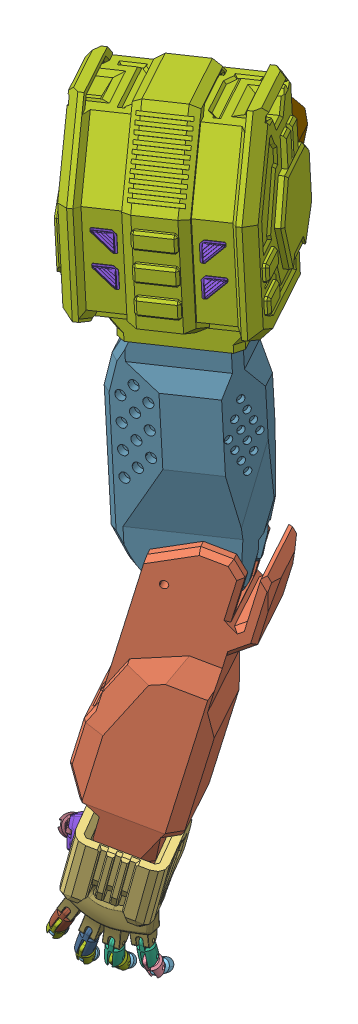
SolidWorks assembly shoulderLEFT, configuration Défaut. Lengths in mm.
Overall size (1126.56 3596.28 1033.18).
88 component instances, 49 part files, 140 mates.
Components (placement in the parent):
- verin_O40intern_050extern_420lenght-1: verin_O40intern_050extern_420lenght [Défaut] at (100 106.457 -34.0488) x (1 0 0) z (0 -0.340071 0.9404)
- épaul1_segment_40x80_0-2: épaul1_segment_40x80_0 [Défaut] at (67.1701 32 -84.1913) x (-0.869368 0 0.494166) z (-0.494166 0 -0.869368) size (40 535 80)
- axeO25_L250-3: axeO25_L250 [Défaut] at (145.1546 609.5 -82.5087) x (0.428557 0.497903 0.753944) z (-0.869368 0 0.494166) size (25 25 310)
- axeO20.25_L250-1: axeO20.25_L250 [Défaut] at (115.5328 92 -65.6711) x (-0.173682 0.936201 -0.305552) z (-0.869368 0 0.494166) size (20 20 80)
- axeO20.25_L250-2: axeO20.25_L250 [Défaut] at (108.4323 515.6503 109.8165) x (-0.45068 -0.410188 -0.792864) z (-0.869368 0 0.494166) size (20 20 80)
- épaul2_segment_40x80_0-1: épaul2_segment_40x80_0 [Défaut] at (-133.5936 647.7925 28.0432) x (-0.869368 0 0.494166) z (-0.020662 0.999125 -0.036351) size (40 300 80)
- épaul2_segment_40x80_0-2: épaul2_segment_40x80_0 [Défaut] at (127.2167 647.7925 -120.2065) x (-0.869368 0 0.494166) z (-0.020662 0.999125 -0.036351) size (40 300 80)
- épaul1_segment_40x80_1-1: épaul1_segment_40x80_1 [Défaut] at (-37.154 -55.5 -24.8914) x (-0.869368 0 0.494166) z (-0.494166 0 -0.869368) size (40 209.28 80)
- épaul1_segment_40x80_1-2: épaul1_segment_40x80_1 [Défaut] at (37.154 -55.5 24.8914) x (0.869368 0 -0.494166) z (0.494166 0 0.869368) size (40 209.28 80)
- épaul1_segment_40x80_0-4: épaul1_segment_40x80_0 [Défaut] at (-67.1701 32 84.1913) x (0.869368 0 -0.494166) z (0.494166 0 0.869368) size (40 535 80)
- épaul1_segment_40x80_2-1: épaul1_segment_40x80_2 [Défaut] at (2.3793 -55.5 44.658) x (0.869368 0 -0.494166) z (0.494166 0 0.869368) size (40 80 80)
- épaul2_segment_40x80_1-1: épaul2_segment_40x80_1 [Défaut] at (16.1794 580.4063 291.5335) x (-0.493734 -0.041813 -0.868607) z (0.020662 -0.999125 0.036351) size (40 260 80)
- épaul2_segment_40x80_3-1: épaul2_segment_40x80_3 [Défaut] at (43.2297 515.6503 146.8789) x (0.362675 -0.679243 0.638041) z (0.869368 0 -0.494166) size (84.94 190.38 10)
- épaul2_segment_40x80_3-2: épaul2_segment_40x80_3 [Défaut] at (95.3918 515.6503 117.229) x (0.362675 -0.679243 0.638041) z (0.869368 0 -0.494166) size (84.94 190.38 10)
- Cylindre_O40intern_050extern_420lenght-1: Cylindre_O40intern_050extern_420lenght [Défaut] at (2.8702 108.5081 5.0494) x (-0.869368 0 0.494166) z (-0.466155 0.331891 -0.82009) size (52 385 57)
- TigeO25_pistonO40-1: TigeO25_pistonO40 [Défaut] at (16.6198 187.5905 29.2385) x (0.869368 0 -0.494166) z (0.466155 -0.331891 0.82009) size (40 367.9 40.25)
- 010.20.0314.001.5111_extern-1: 010.20.0314.001.5111_extern [Défaut] at origin size (386 44 386)
- 010.20.0314.001.5111_intern-1: 010.20.0314.001.5111_intern [Défaut] x (0.869368 0 -0.494166) z (0.494166 0 0.869368) size (310 44 310)
- épaul2_fixation_3-1: épaul2_fixation_3 [Défaut] at (0 32 0) x (0 1 0) z (-0.869368 0 0.494166) size (10 312 312)
- coude-3: coude [Défaut] at (220.7986 -775.7872 464.0221) x (0.132355 0.970732 -0.200406) z (0.49109 0.111404 0.863956)
- attache_verin_cokpitepaul2-1: attache_verin_cokpitepaul2 [Défaut] at (89.4624 260 156.7799) x (0.265308 0 -0.964164) z (0 1 0) size (92.03 103.34 10)
- attache_verin_cokpitepaul2-2: attache_verin_cokpitepaul2 [Défaut] at (89.4624 190 156.7799) x (0.265308 0 -0.964164) z (0 1 0) size (92.03 103.34 10)
- 011.20.0342.101.5111_intern-1: 011.20.0342.101.5111_intern [Défaut] at (149.6013 622.1692 263.1881) x (0.020662 -0.999125 0.036351) z (0.869368 0 -0.494166) size (340 43 340)
- 011.20.0342.101.5111_extern-1: 011.20.0342.101.5111_extern [Défaut] at (149.6013 622.1692 263.1881) x (0.282027 0.937157 -0.205422) z (-0.82261 0.346394 0.450913) size (438.28 43 438.28)
- V4_épaul2_segment_40x80_2_motor_attach-1: V4_épaul2_segment_40x80_2_motor_attach [Défaut] at (128.3707 620.3713 225.8379) x (-0.493734 -0.041813 -0.868607) z (-0.020662 0.999125 -0.036351) size (10 539.36 539.36)
- SAUER-DANFOSS OMP-1: SAUER-DANFOSS OMP [080] at (268.8657 799.7919 107.408) x (-0.629346 0.706488 0.323724) z (0.493734 0.041813 0.868607) size (133 106.5 207.3)
  - SAUER-DANFOSS OMP Part_2-1: SAUER-DANFOSS OMP Part_2 [Default] at (0 0 16) size (35 35 55.3)
  - SAUER-DANFOSS OMP Part_1-2: SAUER-DANFOSS OMP Part_1 [080] at origin size (133 106.5 160)
- SAUER-DANFOSS OMP-2: SAUER-DANFOSS OMP [080] at (276.3316 438.7764 120.5426) x (0.600125 0.706488 -0.375132) z (0.493734 0.041813 0.868607) size (133 106.5 207.3)
  - SAUER-DANFOSS OMP Part_2-1: SAUER-DANFOSS OMP Part_2 [Default] at (0 0 16) size (35 35 55.3)
  - SAUER-DANFOSS OMP Part_1-2: SAUER-DANFOSS OMP Part_1 [080] at origin size (133 106.5 160)
- SAUER-DANFOSS OMP-3: SAUER-DANFOSS OMP [080] at (-45.2643 799.7919 285.9657) x (-0.600125 -0.706488 0.375132) z (0.493734 0.041813 0.868607) size (133 106.5 207.3)
  - SAUER-DANFOSS OMP Part_2-1: SAUER-DANFOSS OMP Part_2 [Default] at (0 0 16) size (35 35 55.3)
  - SAUER-DANFOSS OMP Part_1-2: SAUER-DANFOSS OMP Part_1 [080] at origin size (133 106.5 160)
- SAUER-DANFOSS OMP-4: SAUER-DANFOSS OMP [080] at (-37.7984 438.7764 299.1003) x (0.629346 -0.706488 -0.323724) z (0.493734 0.041813 0.868607) size (133 106.5 207.3)
  - SAUER-DANFOSS OMP Part_2-1: SAUER-DANFOSS OMP Part_2 [Default] at (0 0 16) size (35 35 55.3)
  - SAUER-DANFOSS OMP Part_1-2: SAUER-DANFOSS OMP Part_1 [080] at origin size (133 106.5 160)
- driving gear_modul5_Z17-1: driving gear_modul5_Z17 [Défaut] at (285.1589 801.1718 136.072) x (-0.083872 0.996477 -0.000294) z (0.865559 0.072706 -0.495501) size (94.56 40 94.56)
- driving gear_modul5_Z17-2: driving gear_modul5_Z17 [Défaut] at (-28.9711 801.1718 314.6297) x (-0.147931 0.988324 0.036511) z (0.856939 0.14652 -0.494154) size (94.56 40 94.56)
- driving gear_modul5_Z17-3: driving gear_modul5_Z17 [Défaut] at (292.6248 440.1562 149.2067) x (-0.306737 0.943017 0.128961) z (0.81372 0.330106 -0.478425) size (94.56 40 94.56)
- driving gear_modul5_Z17-4: driving gear_modul5_Z17 [Défaut] at (-21.5052 440.1562 327.7643) x (-0.835862 0.298393 0.460756) z (0.239921 0.953527 -0.182276) size (94.56 40 94.56)
- épaule_bras1-1: épaule_bras1 [Défaut] at (153.0574 622.4619 269.2683) x (0.866867 0.055647 -0.495423) z (0.493734 0.041813 0.868607) size (500 630 10)
- epaul_poutre40x40x180-1: epaul_poutre40x40x180 [Défaut] at (336.4806 614.1964 165.4048) x (0.866867 0.055647 -0.495423) z (0.493734 0.041813 0.868607) size (40 40 180)
- epaul_poutre40x40x180-2: epaul_poutre40x40x180 [Défaut] at (-62.2784 588.5986 393.2995) x (0.866867 0.055647 -0.495423) z (0.493734 0.041813 0.868607) size (40 40 180)
- epaul_poutre40x40x180-3: epaul_poutre40x40x180 [Défaut] at (121.2194 830.8396 277.3348) x (0.866867 0.055647 -0.495423) z (0.493734 0.041813 0.868607) size (40 40 180)
- épaule_bras2-1: épaule_bras2 [Défaut] at (236.9921 629.5701 416.9316) x (0.866867 0.055647 -0.495423) z (0.493734 0.041813 0.868607) size (500 630 10)
- épaule_bras3-1: épaule_bras3 [Défaut] at (0 42 0) x (0.494166 0 0.869368) z (-0.869368 0 0.494166) size (312 480 312)
- decobras2_epaulièreV2LEFT-1: decobras2_epaulièreV2LEFT [Défaut] at (655.9391 173.3724 1098.7432) x (-0.866867 -0.055647 0.495423) z (-0.493734 -0.041813 -0.868607) size (700 900 550)
- airvent-1: airvent [Défaut] at (462.823 534.1597 534.9239) x (0.069051 -0.997575 0.008771) z (-0.866867 -0.055647 0.495423) size (85 14 85)
- airvent-2: airvent [Défaut] at (224.9935 649.1535 664.5754) x (-0.866867 -0.055647 0.495423) z (-0.069051 0.997575 -0.008771) size (85 14 85)
- airvent-3: airvent [Défaut] at (453.8465 663.8444 533.7837) x (0.069051 -0.997575 0.008771) z (-0.866867 -0.055647 0.495423) size (85 14 85)
- airvent-4: airvent [Défaut] at (233.97 519.4689 665.7157) x (-0.866867 -0.055647 0.495423) z (-0.069051 0.997575 -0.008771) size (85 14 85)
- airvent-5: airvent [Défaut] at (18.9919 762.7172 696.3533) x (-0.493734 -0.041813 -0.868607) z (-0.069051 0.997575 -0.008771) size (85 14 85)
- decobras3_epaulmid-1: decobras3_epaulmid [Défaut] at (128.3707 620.3713 225.8379) x (-0.493734 -0.041813 -0.868607) z (0.869368 0 -0.494166) size (320 535.44 535.44)
- bras(haut)-1: bras(haut) [Défaut] at (391.8676 539.4125 344.7499) x (-0.866867 -0.055647 0.495423) z (-0.493734 -0.041813 -0.868607) size (510 1200 300)
  - humerusV2-1: humerusV2 [Défaut] at origin size (330 1200 180)
  - axeO30_L250-1: axeO30_L250 [Défaut] at (240 -1240 -20) x (0.999987 0.005029 0) z (0 0 1) size (30 30 220)
  - humerus_attache vérin-1: humerus_attache vérin [Défaut] at (290 -632.1214 40) x (0 -1 0) z (0 0 -1) size (207.88 83.56 10)
  - humerus_attache vérin-2: humerus_attache vérin [Défaut] at (290 -632.1214 150) x (0 -1 0) z (0 0 -1) size (207.88 83.56 10)
  - axeO20.25_L150-1: axeO20.25_L150 [Défaut] at (237.9719 -695.6462 144.2274) x (-0.412113 0.911133 0) z (0 0 -1) size (20.25 20.25 110)
  - decobras5_bras-1: decobras5_bras [Défaut] at (440 -1280 90) x (0 0 -1) z (1 0 0) size (300 890 510)
- 2Cylindre_O40intern_050extern_420lenght-2: 2Cylindre_O40intern_050extern_420lenght [Défaut] at (192.7619 -188.6376 389.358) x (0.493734 0.041813 0.868607) z (0.845132 0.212262 -0.490608) size (52 385 57)
- 2TigeO25_pistonO40-2: 2TigeO25_pistonO40 [Défaut] at (205.6573 -250.0867 384.986) x (0.493734 0.041813 0.868607) z (0.845132 0.212262 -0.490608) size (40 367.9 40.25)
- Avant bras-1: Avant bras [Défaut] at (294.6244 -810.3538 401.6797) x (0.193576 0.968498 -0.156653) z (0.493734 0.041813 0.868607) size (1290.18 220 110)
  - coude2-1: coude2 [Défaut] at origin size (290 120 10)
  - coude2-2: coude2 [Défaut] at (0 0 -80) size (290 120 10)
  - coude3-1: coude3 [Défaut] at (0 0 10) size (290 10 90)
  - axeO20.25_L150-1: axeO20.25_L150 [Défaut] at (216.7479 50 -90) x (0.918259 -0.39598 0) z (0 0 1) size (20.25 20.25 110)
  - avantbras-1: avantbras [Défaut] at (370.8246 -100 -85) x (0 0 1) z (0 -1 0) size (100 1290.18 100)
- decobras6_avantbras-1: decobras6_avantbras [Défaut] at (-175.3127 -1751.4903 385.9938) x (0.847795 -0.245487 -0.470086) z (0.493734 0.041813 0.868607) size (440 1250 390)
- decobras6_poignéLEFT-1: decobras6_poignéLEFT [Défaut] at (20.069 -1562.5613 522.7007) x (0.847795 -0.245487 -0.470086) z (-0.30663 -0.950131 -0.056829) size (310 305 300)
- mecha_hand_LEFT-1: mecha_hand_LEFT [Défaut] at (64.4874 -1911.8509 472.2207) x (0.728033 -0.668928 -0.150012) z (0.623184 0.736956 -0.261797) size (666.05 313.23 634.37)
  - FA02-1: FA02 [Défaut] at (318.8479 -0.9351 -108.5088) x (0.342871 -0.229443 0.910931) z (-0.847095 -0.494671 0.194246) size (95.83 71.04 113.76)
  - FA03-1: FA03 [Défaut] at (352.5482 26.9146 -138.6421) x (0.487616 -0.389848 0.781184) z (-0.535029 -0.840498 -0.085483) size (78.66 63.16 106.66)
  - FA04-1: FA04 [Défaut] at (210.1629 -21.1941 -197.1885) x (0.68922 -0.05924 0.722126) z (-0.706133 -0.278215 0.651132) size (76.15 64.38 116.68)
  - FA05-1: FA05 [Défaut] at (236.6434 -1.1911 -234.8244) x (0.722438 -0.152852 0.674329) z (-0.550129 -0.71786 0.426657) size (80.78 65.45 124.81)
  - FA03-2: FA03 [Défaut] at (284.0518 44.6888 -254.044) x (0.628724 -0.368149 0.684962) z (-0.596116 -0.793801 0.120525) size (78.66 63.16 106.66)
  - FA05-2: FA05 [Défaut] at (160.9262 -12.3117 -298.7683) x (0.829813 -0.113657 0.546345) z (-0.514802 -0.533784 0.67086) size (80.78 65.45 124.81)
  - FA03-3: FA03 [Défaut] at (207.699 21.223 -336.813) x (0.752271 -0.366879 0.547255) z (-0.561853 -0.791041 0.242024) size (78.66 63.16 106.66)
  - FA05-3: FA05 [Défaut] at (57.436 -6.8266 -327.3227) x (0.921377 -0.101426 0.375202) z (-0.376082 -0.476338 0.794773) size (80.78 65.45 124.81)
  - FA03-4: FA03 [Défaut] at (96.0618 22.8503 -376.3263) x (0.846841 -0.366169 0.385721) z (-0.502126 -0.789505 0.35292) size (78.66 63.16 106.66)
  - PA02-1: PA02 [Défaut] at (-92.7063 -27.7729 -93.6202) x (-0.864558 0.32477 -0.383491) z (-0.383491 0.066797 0.921126) size (137.04 69.48 175.33)
  - POL03-1: POL03 [Défaut] at (-193.4912 128.4807 -56.1901) x (0.563945 -0.434468 -0.702285) z (0.555335 -0.429893 0.711895) size (78.15 141.82 81.12)
  - FA07-1: FA07 [Défaut] at (48.7036 -25.842 -285.2347) x (0.978633 0.029631 0.20347) z (-0.197253 -0.144068 0.969709) size (75.62 64.39 118.37)
  - FA08-1: FA08 [Défaut] at (-43.1637 -22.0262 -299.5212) x (0.979497 0 0.201457) z (-0.195554 -0.240299 0.950797) size (63.71 64.39 113.98)
  - FA04-2: FA04 [Défaut] at (262.7159 -19.9252 -96.0309) x (0.503834 -0.057708 0.86187) z (-0.838795 -0.271021 0.472198) size (76.15 64.38 116.68)
  - mech_hand_LEFT-1: mech_hand_LEFT [Défaut] at (-270.8385 -50.9556 -169.053) size (425.79 104.09 449.81)
  - POL02_LEFT-2: POL02_LEFT [Défaut] at (-96.686 -97.2472 -120.1216) x (-0.209537 -0.572925 0.792371) z (-0.630903 0.698325 0.338087) size (166.06 83.76 109.31)
Mates (geometry in assembly coordinates):
- Coaxiale9: concentric anti-aligned: cylinder of ? through (120 504.011 109.7163) axis (-1 0 0) radius 10.125; cylinder of axeO20.25_L250-2 through (-9.5877 504.011 109.7163) axis (1 0 0) radius 10.125
- Coaxiale11: concentric aligned: cylinder of verin_O40intern_050extern_420lenght-1 through (74 90 -40) axis (1 0 0) radius 10.125; cylinder of axeO20.25_L250-1 through (-19.5771 90 -40) axis (1 0 0) radius 10.125
- Coaxiale12: concentric anti-aligned: cylinder of épaul1_segment_40x80_0-2 through (86.9368 92 -49.4166) axis (-0.869368 0 0.494166) radius 10.125; cylinder of axeO20.25_L250-1 through (45.9834 92 -26.1378) axis (0.869368 0 -0.494166) radius 10
- Coaxiale14: concentric anti-aligned: cylinder of axeO25_L250-3 through (-124.3494 609.5 70.6827) axis (0.869368 0 -0.494166) radius 12.5; cylinder of épaul2_segment_40x80_0-2 through (147.7925 609.5 -84.0082) axis (-0.869368 0 0.494166) radius 12.5
- Coaxiale15: concentric anti-aligned: cylinder of axeO25_L250-3 through (-124.3494 609.5 70.6827) axis (0.869368 0 -0.494166) radius 12.5; cylinder of épaul2_segment_40x80_0-1 through (-113.0178 609.5 64.2415) axis (-0.869368 0 0.494166) radius 12.5
- Coïncidente6: coincident aligned: plane of épaul2_segment_40x80_0-1 through (14.4407 580.4063 292.5218) normal (0.020662 -0.999125 0.036351); plane of épaul2_segment_40x80_0-2 through (275.251 580.4063 144.2721) normal (0.020662 -0.999125 0.036351)
- Distance11: distance = 35 mm anti-aligned: plane of épaul1_segment_40x80_0-2; cylinder of verin_O40intern_050extern_420lenght-1 through (100 109.2782 -33.0285) axis (0 -0.9404 -0.340071) radius 25
- Coïncidente15: coincident anti-aligned: plane of épaul1_segment_40x80_0-2 through (33.3838 707 -62.6859) normal (-0.869368 0 0.494166); plane of épaul1_segment_40x80_1-2 through (70.9404 649.5 3.386) normal (0.869368 0 -0.494166)
- Coïncidente17: coincident aligned: plane of épaul1_segment_40x80_0-2 through (65.4314 707 -83.2029) normal (-0.494166 0 -0.869368); plane of épaul1_segment_40x80_1-2 through (-0.6405 649.5 -45.6464) normal (-0.494166 0 -0.869368)
- Coaxiale19: concentric aligned: cylinder of axeO25_L250-3 through (-124.3494 609.5 70.6827) axis (0.869368 0 -0.494166) radius 12.5; cylinder of épaul1_segment_40x80_1-2 through (17.3874 609.5 -9.8833) axis (0.869368 0 -0.494166) radius 12.5
- Coïncidente20: coincident aligned: plane of épaul1_segment_40x80_1-1 through (-37.9044 649.5 -22.1643) normal (0 1 0); plane of épaul1_segment_40x80_1-2 through (37.9044 649.5 22.1643) normal (0 1 0)
- Coïncidente24: coincident anti-aligned: plane of épaul1_segment_40x80_1-1 through (-70.9404 649.5 -3.386) normal (-0.869368 0 0.494166); plane of épaul1_segment_40x80_0-4 through (-33.3838 707 62.6859) normal (0.869368 0 -0.494166)
- Coïncidente25: coincident aligned: plane of épaul1_segment_40x80_1-1 through (-38.8927 649.5 -23.9031) normal (-0.494166 0 -0.869368); plane of épaul1_segment_40x80_0-4 through (-104.9647 707 13.6535) normal (-0.494166 0 -0.869368)
- Coïncidente26: coincident aligned: plane of épaul1_segment_40x80_0-2 through (66.4197 32 -81.4642) normal (0 -1 0); plane of épaul1_segment_40x80_0-4 through (-66.4197 32 81.4642) normal (0 -1 0)
- Coaxiale21: concentric aligned: cylinder of axeO20.25_L250-1 through (45.9834 92 -26.1378) axis (0.869368 0 -0.494166) radius 10; cylinder of épaul1_segment_40x80_0-4 through (-86.9368 92 49.4166) axis (0.869368 0 -0.494166) radius 10.125
- Distance15: distance = 35 mm anti-aligned: cylinder of verin_O40intern_050extern_420lenght-1 through (100 109.2782 -33.0285) axis (0 -0.9404 -0.340071) radius 25; plane of 010.20.0314.001.5111_extern-1
- Coïncidente32: coincident aligned: plane of épaul1_segment_40x80_1-1 through (-38.8927 649.5 -23.9031) normal (-0.494166 0 -0.869368); plane of épaul1_segment_40x80_2-1 through (-35.4152 649.5 -25.8797) normal (-0.494166 0 -0.869368)
- Coïncidente33: coincident aligned: plane of épaul1_segment_40x80_1-1 through (-37.9044 649.5 -22.1643) normal (0 1 0); plane of épaul1_segment_40x80_2-1 through (3.1297 649.5 41.931) normal (0 1 0)
- Coïncidente34: coincident anti-aligned: plane of épaul1_segment_40x80_1-2 through (36.1657 649.5 23.1527) normal (-0.869368 0 0.494166); plane of épaul1_segment_40x80_2-1 through (36.1657 649.5 23.1527) normal (0.869368 0 -0.494166)
- Distance17: distance = 70 mm anti-aligned: plane of épaul1_segment_40x80_1-2 through (70.9404 649.5 3.386) normal (0.869368 0 -0.494166); plane of épaul2_segment_40x80_0-2 through (240.6034 658.3381 160.2151) normal (-0.869368 0 0.494166)
- Distance18: distance = 70 mm anti-aligned: plane of épaul1_segment_40x80_1-1 through (-70.9404 649.5 -3.386) normal (-0.869368 0 0.494166); plane of épaul2_segment_40x80_0-1 through (14.5678 658.3381 288.6982) normal (0.869368 0 -0.494166)
- Coïncidente41: coincident aligned: plane of épaul2_segment_40x80_0-2 through (273.598 660.3363 141.3641) normal (-0.020662 0.999125 -0.036351); plane of épaul2_segment_40x80_1-1 through (239.5746 660.2527 158.4051) normal (-0.020662 0.999125 -0.036351)
- Coïncidente42: coincident anti-aligned: plane of épaul2_segment_40x80_0-2 through (240.6034 658.3381 160.2151) normal (-0.869368 0 0.494166); plane of épaul2_segment_40x80_1-1 through (241.1862 582.3209 161.2405) normal (0.869368 0 -0.494166)
- Coïncidente46: coincident anti-aligned: plane of épaul2_segment_40x80_1-1 through (222.4244 580.732 128.2334) normal (-0.493734 -0.041813 -0.868607); plane of épaul2_segment_40x80_3-2 through (139.8757 578.7338 175.2519) normal (0.493734 0.041813 0.868607)
- Coïncidente47: coincident anti-aligned: plane of épaul2_segment_40x80_1-1 through (241.2276 580.3226 161.3132) normal (0.020662 -0.999125 0.036351); plane of épaul2_segment_40x80_3-2 through (159.6251 580.4063 209.9962) normal (-0.020662 0.999125 -0.036351)
- Coaxiale23: concentric anti-aligned: cylinder of axeO20.25_L250-2 through (38.8829 515.6503 149.3498) axis (0.869368 0 -0.494166) radius 10; cylinder of épaul2_segment_40x80_3-2 through (104.0855 515.6503 112.2873) axis (-0.869368 0 0.494166) radius 23.5
- Coïncidente48: coincident anti-aligned: plane of épaul2_segment_40x80_1-1 through (222.4244 580.732 128.2334) normal (-0.493734 -0.041813 -0.868607); plane of épaul2_segment_40x80_3-1 through (87.7137 578.7338 204.9018) normal (0.493734 0.041813 0.868607)
- Coïncidente49: coincident anti-aligned: plane of épaul2_segment_40x80_1-1 through (241.2276 580.3226 161.3132) normal (0.020662 -0.999125 0.036351); plane of épaul2_segment_40x80_3-1 through (107.463 580.4063 239.6461) normal (-0.020662 0.999125 -0.036351)
- Coaxiale24: concentric anti-aligned: cylinder of axeO20.25_L250-2 through (38.8829 515.6503 149.3498) axis (0.869368 0 -0.494166) radius 10; cylinder of TigeO25_pistonO40-1 through (91.045 515.6503 119.6998) axis (-0.869368 0 0.494166) radius 10.125
- Coaxiale25: concentric aligned: cylinder of Cylindre_O40intern_050extern_420lenght-1 through (3.3622 111.338 5.915) axis (-0.164009 -0.943318 -0.288535) radius 25; cylinder of TigeO25_pistonO40-1 through (16.6198 187.5905 29.2385) axis (-0.164009 -0.943318 -0.288535) radius 12.5
- Coaxiale26: concentric anti-aligned: cylinder of axeO20.25_L250-1 through (45.9834 92 -26.1378) axis (0.869368 0 -0.494166) radius 10; cylinder of Cylindre_O40intern_050extern_420lenght-1 through (22.6036 92 -12.8483) axis (-0.869368 0 0.494166) radius 10.125
- Distance19: distance = 35 mm anti-aligned: cylinder of Cylindre_O40intern_050extern_420lenght-1 through (3.3622 111.338 5.915) axis (-0.164009 -0.943318 -0.288535) radius 25; plane of épaul1_segment_40x80_0-2 through (33.3838 707 -62.6859) normal (-0.869368 0 0.494166)
- Distance20: distance = 35 mm anti-aligned: cylinder of Cylindre_O40intern_050extern_420lenght-1 through (3.3622 111.338 5.915) axis (-0.164009 -0.943318 -0.288535) radius 25; plane of épaul1_segment_40x80_0-4 through (-33.3838 707 62.6859) normal (0.869368 0 -0.494166)
- Distance25: distance = 495 mm: cylinder of axeO25_L250-3 through (-124.3494 609.5 70.6827) axis (0.869368 0 -0.494166) radius 12.5; cylinder of axeO20.25_L250-1 through (45.9834 92 -26.1378) axis (0.869368 0 -0.494166) radius 10
- Coaxiale32: concentric aligned: cylinder of 010.20.0314.001.5111_extern-1 through (0 44 0) axis (0 1 0) radius 193; cylinder of 010.20.0314.001.5111_intern-1 through (0 44 0) axis (0 1 0) radius 155
- Coïncidente52: coincident aligned: plane of 010.20.0314.001.5111_extern-1 through (0 0 0) normal (0 -1 0); plane of 010.20.0314.001.5111_intern-1 through (-134.752 0 76.5957) normal (0 -1 0)
- Coïncidente53: coincident anti-aligned: plane of 010.20.0314.001.5111_intern-1 through (-134.752 32 76.5957) normal (0 1 0); plane of épaul2_fixation_3-1 through (0 32 0) normal (0 -1 0)
- Coaxiale33: concentric anti-aligned: cylinder of 010.20.0314.001.5111_intern-1 through (-66.2182 -12 -116.4953) axis (0 1 0) radius 6.75; cylinder of épaul2_fixation_3-1 through (-66.2182 42 -116.4953) axis (0 -1 0) radius 6.75
- Coaxiale34: concentric anti-aligned: cylinder of 010.20.0314.001.5111_intern-1 through (66.2182 -12 116.4953) axis (0 1 0) radius 6.75; cylinder of épaul2_fixation_3-1 through (66.2182 42 116.4953) axis (0 -1 0) radius 6.75
- Coïncidente54: coincident anti-aligned: plane of épaul1_segment_40x80_0-4 through (-104.9647 707 13.6535) normal (-0.494166 0 -0.869368); plane of épaul2_fixation_3-1 through (-19.7666 42 -34.7747) normal (0.494166 0 0.869368)
- Coïncidente55: coincident anti-aligned: plane of épaul1_segment_40x80_0-4 through (-33.3838 707 62.6859) normal (0.869368 0 -0.494166); plane of épaul2_fixation_3-1 through (-52.1621 42 29.6499) normal (-0.869368 0 0.494166)
- Coïncidente56: coincident aligned: plane of épaul1_segment_40x80_0-4 through (-66.4197 32 81.4642) normal (0 -1 0); plane of épaul2_fixation_3-1 through (0 32 0) normal (0 -1 0)
- Coïncidente95: coincident anti-aligned: plane of épaul1_segment_40x80_0-4 through (-104.9647 707 13.6535) normal (-0.494166 0 -0.869368); plane of attache_verin_cokpitepaul2-1 through (-106.7034 270 14.6419) normal (0.494166 0 0.869368)
- Coïncidente96: coincident anti-aligned: plane of épaul1_segment_40x80_0-4 through (-68.1585 707 82.4525) normal (-0.869368 0 0.494166); plane of attache_verin_cokpitepaul2-1 through (-106.7034 270 14.6419) normal (0.869368 0 -0.494166)
- Coïncidente97: coincident anti-aligned: plane of épaul1_segment_40x80_0-4 through (-104.9647 707 13.6535) normal (-0.494166 0 -0.869368); plane of attache_verin_cokpitepaul2-2 through (-106.7034 200 14.6419) normal (0.494166 0 0.869368)
- Coïncidente98: coincident anti-aligned: plane of épaul1_segment_40x80_0-4 through (-68.1585 707 82.4525) normal (-0.869368 0 0.494166); plane of attache_verin_cokpitepaul2-2 through (-106.7034 200 14.6419) normal (0.869368 0 -0.494166)
- Distance45: distance = 148 mm anti-aligned: plane of épaul2_fixation_3-1 through (0 42 0) normal (0 1 0); plane of attache_verin_cokpitepaul2-2 through (-143.8237 190 4.4275) normal (0 -1 0)
- Distance46: distance = 60 mm anti-aligned: plane of attache_verin_cokpitepaul2-2 through (-143.8237 200 4.4275) normal (0 1 0); plane of attache_verin_cokpitepaul2-1 through (-143.8237 260 4.4275) normal (0 -1 0)
- Distance47: distance = 50 mm anti-aligned: plane of épaul2_segment_40x80_3-2 through (95.3918 515.6503 117.229) normal (-0.869368 0 0.494166); plane of épaul2_segment_40x80_3-1 through (51.9234 515.6503 141.9373) normal (0.869368 0 -0.494166)
- Distance48: distance = 5 mm anti-aligned: plane of épaul2_segment_40x80_3-1 through (51.9234 515.6503 141.9373) normal (0.869368 0 -0.494166); plane of TigeO25_pistonO40-1 through (56.2703 515.6503 139.4665) normal (-0.869368 0 0.494166)
- Distance49: distance = 5 mm aligned: plane of axeO20.25_L250-2 through (38.8829 515.6503 149.3498) normal (-0.869368 0 0.494166); plane of épaul2_segment_40x80_3-1 through (43.2297 515.6503 146.8789) normal (-0.869368 0 0.494166)
- Coïncidente105: coincident anti-aligned: plane of épaul2_segment_40x80_0-2 through (273.598 660.3363 141.3641) normal (-0.020662 0.999125 -0.036351); plane of V4_épaul2_segment_40x80_2_motor_attach-1 through (235.6247 659.9182 151.4563) normal (0.020662 -0.999125 0.036351)
- Coïncidente106: coincident anti-aligned: plane of épaul2_segment_40x80_0-2 through (275.3781 658.3381 140.4484) normal (0.869368 0 -0.494166); plane of V4_épaul2_segment_40x80_2_motor_attach-1 through (270.3994 659.9182 131.6897) normal (-0.869368 0 0.494166)
- Coïncidente108: coincident aligned: plane of épaul2_segment_40x80_1-1 through (242.1737 582.4045 162.9777) normal (0.493734 0.041813 0.868607); plane of V4_épaul2_segment_40x80_2_motor_attach-1 through (128.3707 620.3713 225.8379) normal (0.493734 0.041813 0.868607)
- Coïncidente109: coincident aligned: plane of épaul2_segment_40x80_0-2 through (273.6393 658.3381 141.4368) normal (0.493734 0.041813 0.868607); plane of V4_épaul2_segment_40x80_2_motor_attach-1 through (128.3707 620.3713 225.8379) normal (0.493734 0.041813 0.868607)
- Coaxiale47: concentric aligned: cylinder of 011.20.0342.101.5111_intern-1 through (128.3707 620.3713 225.8379) axis (-0.493734 -0.041813 -0.868607) radius 132.5; cylinder of 011.20.0342.101.5111_extern-1 through (128.3707 620.3713 225.8379) axis (-0.493734 -0.041813 -0.868607) radius 172
- Coïncidente110: coincident aligned: plane of 011.20.0342.101.5111_intern-1 through (128.3762 787.5179 225.8476) normal (-0.493734 -0.041813 -0.868607); plane of 011.20.0342.101.5111_extern-1 through (131.8269 620.664 231.9182) normal (-0.493734 -0.041813 -0.868607)
- Coaxiale48: concentric anti-aligned: cylinder of 011.20.0342.101.5111_intern-1 through (135.1597 476.1709 278.4249) axis (-0.493734 -0.041813 -0.868607) radius 6.75; cylinder of V4_épaul2_segment_40x80_2_motor_attach-1 through (108.9918 473.9548 232.3887) axis (0.493734 0.041813 0.868607) radius 6.75
- Coaxiale49: concentric anti-aligned: cylinder of 011.20.0342.101.5111_intern-1 through (170.0815 476.1709 258.5747) axis (-0.493734 -0.041813 -0.868607) radius 6.75; cylinder of V4_épaul2_segment_40x80_2_motor_attach-1 through (143.9136 473.9548 212.5385) axis (0.493734 0.041813 0.868607) radius 6.75
- Coïncidente111: coincident anti-aligned: plane of 011.20.0342.101.5111_intern-1 through (124.8581 790.2226 219.6583) normal (-0.493734 -0.041813 -0.868607); plane of V4_épaul2_segment_40x80_2_motor_attach-1 through (128.3707 620.3713 225.8379) normal (0.493734 0.041813 0.868607)
- Coaxiale50: concentric anti-aligned: cylinder of V4_épaul2_segment_40x80_2_motor_attach-1 through (276.7654 800.461 121.3057) axis (0.493734 0.041813 0.868607) radius 41.5; cylinder of SAUER-DANFOSS OMP-1/SAUER-DANFOSS OMP Part_1-2 through (342.2703 806.0083 236.5461) axis (-0.493734 -0.041813 -0.868607) radius 41.25
- Coaxiale51: concentric aligned: cylinder of SAUER-DANFOSS OMP-1/SAUER-DANFOSS OMP Part_1-2 through (310.1208 763.0171 104.1483) axis (0.493734 0.041813 0.868607) radius 6.75; cylinder of V4_épaul2_segment_40x80_2_motor_attach-1 through (310.1208 763.0171 104.1483) axis (0.493734 0.041813 0.868607) radius 6.75
- Coaxiale52: concentric anti-aligned: cylinder of V4_épaul2_segment_40x80_2_motor_attach-1 through (284.2314 439.4454 134.4403) axis (0.493734 0.041813 0.868607) radius 41.5; cylinder of SAUER-DANFOSS OMP-2/SAUER-DANFOSS OMP Part_1-2 through (349.7363 444.9928 249.6807) axis (-0.493734 -0.041813 -0.868607) radius 41.25
- Coaxiale53: concentric aligned: cylinder of SAUER-DANFOSS OMP-2/SAUER-DANFOSS OMP Part_1-2 through (252.4247 402.0015 154.3223) axis (0.493734 0.041813 0.868607) radius 6.75; cylinder of V4_épaul2_segment_40x80_2_motor_attach-1 through (252.4247 402.0015 154.3223) axis (0.493734 0.041813 0.868607) radius 6.75
- Coaxiale54: concentric anti-aligned: cylinder of V4_épaul2_segment_40x80_2_motor_attach-1 through (-29.8986 439.4454 312.998) axis (0.493734 0.041813 0.868607) radius 41.5; cylinder of SAUER-DANFOSS OMP-4/SAUER-DANFOSS OMP Part_1-2 through (35.6063 444.9928 428.2384) axis (-0.493734 -0.041813 -0.868607) radius 41.25
- Coaxiale55: concentric aligned: cylinder of SAUER-DANFOSS OMP-4/SAUER-DANFOSS OMP Part_1-2 through (-63.254 476.8893 330.1554) axis (0.493734 0.041813 0.868607) radius 6.75; cylinder of V4_épaul2_segment_40x80_2_motor_attach-1 through (-63.254 476.8893 330.1554) axis (0.493734 0.041813 0.868607) radius 6.75
- Coaxiale56: concentric anti-aligned: cylinder of V4_épaul2_segment_40x80_2_motor_attach-1 through (-37.3646 800.461 299.8634) axis (0.493734 0.041813 0.868607) radius 41.5; cylinder of SAUER-DANFOSS OMP-3/SAUER-DANFOSS OMP Part_1-2 through (28.1403 806.0083 415.1038) axis (-0.493734 -0.041813 -0.868607) radius 41.25
- Coaxiale57: concentric aligned: cylinder of SAUER-DANFOSS OMP-3/SAUER-DANFOSS OMP Part_1-2 through (-5.558 837.9048 279.9814) axis (0.493734 0.041813 0.868607) radius 6.75; cylinder of V4_épaul2_segment_40x80_2_motor_attach-1 through (-5.558 837.9048 279.9814) axis (0.493734 0.041813 0.868607) radius 6.75
- Coïncidente112: coincident anti-aligned: plane of V4_épaul2_segment_40x80_2_motor_attach-1 through (123.4334 619.9532 217.1519) normal (-0.493734 -0.041813 -0.868607); plane of SAUER-DANFOSS OMP-3/SAUER-DANFOSS OMP Part_1-2 through (-37.3646 800.461 299.8634) normal (0.493734 0.041813 0.868607)
- Coïncidente113: coincident anti-aligned: plane of V4_épaul2_segment_40x80_2_motor_attach-1 through (123.4334 619.9532 217.1519) normal (-0.493734 -0.041813 -0.868607); plane of SAUER-DANFOSS OMP-4/SAUER-DANFOSS OMP Part_1-2 through (-29.8986 439.4454 312.998) normal (0.493734 0.041813 0.868607)
- Coïncidente114: coincident anti-aligned: plane of V4_épaul2_segment_40x80_2_motor_attach-1 through (123.4334 619.9532 217.1519) normal (-0.493734 -0.041813 -0.868607); plane of SAUER-DANFOSS OMP-1/SAUER-DANFOSS OMP Part_1-2 through (276.7654 800.461 121.3057) normal (0.493734 0.041813 0.868607)
- Coïncidente115: coincident anti-aligned: plane of V4_épaul2_segment_40x80_2_motor_attach-1 through (123.4334 619.9532 217.1519) normal (-0.493734 -0.041813 -0.868607); plane of SAUER-DANFOSS OMP-2/SAUER-DANFOSS OMP Part_1-2 through (284.2314 439.4454 134.4403) normal (0.493734 0.041813 0.868607)
- Coaxiale58: concentric aligned: cylinder of SAUER-DANFOSS OMP-1/SAUER-DANFOSS OMP Part_2-1 through (276.7654 800.461 121.3057) axis (0.493734 0.041813 0.868607) radius 12.7; cylinder of driving gear_modul5_Z17-1 through (285.1589 801.1718 136.072) axis (0.493734 0.041813 0.868607) radius 12.7
- Coaxiale59: concentric aligned: cylinder of SAUER-DANFOSS OMP-3/SAUER-DANFOSS OMP Part_2-1 through (-37.3646 800.461 299.8634) axis (0.493734 0.041813 0.868607) radius 12.7; cylinder of driving gear_modul5_Z17-2 through (-28.9711 801.1718 314.6297) axis (0.493734 0.041813 0.868607) radius 12.7
- Coaxiale60: concentric aligned: cylinder of SAUER-DANFOSS OMP-2/SAUER-DANFOSS OMP Part_2-1 through (284.2314 439.4454 134.4403) axis (0.493734 0.041813 0.868607) radius 12.7; cylinder of driving gear_modul5_Z17-3 through (292.6248 440.1562 149.2067) axis (0.493734 0.041813 0.868607) radius 12.7
- Coaxiale61: concentric aligned: cylinder of SAUER-DANFOSS OMP-4/SAUER-DANFOSS OMP Part_2-1 through (-29.8986 439.4454 312.998) axis (0.493734 0.041813 0.868607) radius 12.7; cylinder of driving gear_modul5_Z17-4 through (-21.5052 440.1562 327.7643) axis (0.493734 0.041813 0.868607) radius 12.7
- Coïncidente116: coincident aligned: plane of 011.20.0342.101.5111_extern-1 through (131.8269 620.664 231.9182) normal (-0.493734 -0.041813 -0.868607); plane of driving gear_modul5_Z17-4 through (11.9293 428.2205 309.3341) normal (-0.493734 -0.041813 -0.868607)
- Coïncidente117: coincident aligned: plane of 011.20.0342.101.5111_extern-1 through (131.8269 620.664 231.9182) normal (-0.493734 -0.041813 -0.868607); plane of driving gear_modul5_Z17-2 through (-23.0539 761.6388 313.1693) normal (-0.493734 -0.041813 -0.868607)
- Coïncidente118: coincident aligned: plane of 011.20.0342.101.5111_extern-1 through (131.8269 620.664 231.9182) normal (-0.493734 -0.041813 -0.868607); plane of driving gear_modul5_Z17-1 through (288.5137 761.3127 136.0838) normal (-0.493734 -0.041813 -0.868607)
- Coïncidente119: coincident aligned: plane of 011.20.0342.101.5111_extern-1 through (131.8269 620.664 231.9182) normal (-0.493734 -0.041813 -0.868607); plane of driving gear_modul5_Z17-3 through (304.8943 402.4355 144.0482) normal (-0.493734 -0.041813 -0.868607)
- Contr.Engrenages2: gear = 84 : 17 mm: circle of driving gear_modul5_Z17-2; circle of 011.20.0342.101.5111_extern-1
- Contr.Engrenages5: gear = 84 : 17 mm: circle of driving gear_modul5_Z17-1; circle of 011.20.0342.101.5111_extern-1
- Contr.Engrenages6: gear = 84 : 17 mm: circle of driving gear_modul5_Z17-3; circle of 011.20.0342.101.5111_extern-1
- Contr.Engrenages7: gear = 344 : 17 mm: circle of driving gear_modul5_Z17-4; circle of 011.20.0342.101.5111_extern-1
- Coaxiale73: concentric aligned: cylinder of 011.20.0342.101.5111_extern-1 through (139.5925 816.989 267.5579) axis (-0.493734 -0.041813 -0.868607) radius 6.75; cylinder of épaule_bras1-1 through (144.5299 817.4071 276.244) axis (-0.493734 -0.041813 -0.868607) radius 6.75
- Coaxiale74: concentric aligned: cylinder of 011.20.0342.101.5111_extern-1 through (185.6981 812.703 241.557) axis (-0.493734 -0.041813 -0.868607) radius 6.75; cylinder of épaule_bras1-1 through (190.6354 813.1211 250.243) axis (-0.493734 -0.041813 -0.868607) radius 6.75
- Coïncidente140: coincident anti-aligned: plane of 011.20.0342.101.5111_extern-1 through (153.0574 622.4619 269.2683) normal (0.493734 0.041813 0.868607); plane of épaule_bras1-1 through (153.0574 622.4619 269.2683) normal (-0.493734 -0.041813 -0.868607)
- Coïncidente143: coincident aligned: plane of épaule_bras1-1 through (153.0574 622.4619 269.2683) normal (-0.493734 -0.041813 -0.868607); plane of epaul_poutre40x40x180-2 through (-60.6828 590.7051 392.2911) normal (-0.493734 -0.041813 -0.868607)
- Coïncidente144: coincident anti-aligned: plane of épaule_bras1-1 through (-57.3411 589.0167 401.9856) normal (-0.069051 0.997575 -0.008771); plane of epaul_poutre40x40x180-2 through (28.3273 596.2362 548.658) normal (0.069051 -0.997575 0.008771)
- Coïncidente145: coincident anti-aligned: plane of épaule_bras1-1 through (-22.6664 591.2426 382.1687) normal (-0.866867 -0.055647 0.495423); plane of epaul_poutre40x40x180-2 through (61.1302 600.3459 529.8144) normal (0.866867 0.055647 -0.495423)
- Coïncidente146: coincident anti-aligned: plane of épaule_bras1-1 through (338.6559 654.5175 173.7401) normal (0.866867 0.055647 -0.495423); plane of epaul_poutre40x40x180-1 through (425.2145 623.7178 321.7366) normal (-0.866867 -0.055647 0.495423)
- Coïncidente147: coincident anti-aligned: plane of épaule_bras1-1 through (373.3306 656.7434 153.9231) normal (0.069051 -0.997575 0.008771); plane of epaul_poutre40x40x180-1 through (424.3243 661.7369 320.4125) normal (-0.069051 0.997575 -0.008771)
- Coïncidente148: coincident aligned: plane of épaule_bras1-1 through (153.0574 622.4619 269.2683) normal (-0.493734 -0.041813 -0.868607); plane of epaul_poutre40x40x180-1 through (338.0762 616.3028 164.3965) normal (-0.493734 -0.041813 -0.868607)
- Coïncidente149: coincident anti-aligned: plane of épaule_bras1-1 through (123.3947 871.1608 285.6701) normal (0.866867 0.055647 -0.495423); plane of epaul_poutre40x40x180-3 through (209.9534 840.3611 433.6666) normal (-0.866867 -0.055647 0.495423)
- Coïncidente150: coincident anti-aligned: plane of épaule_bras1-1 through (126.1568 831.2578 286.0209) normal (-0.069051 0.997575 -0.008771); plane of epaul_poutre40x40x180-3 through (211.8252 838.4772 432.6933) normal (0.069051 -0.997575 0.008771)
- Coïncidente152: coincident aligned: plane of épaule_bras1-1 through (153.0574 622.4619 269.2683) normal (-0.493734 -0.041813 -0.868607); plane of epaul_poutre40x40x180-3 through (122.8151 832.9461 276.3264) normal (-0.493734 -0.041813 -0.868607)
- Coïncidente153: coincident anti-aligned: plane of epaul_poutre40x40x180-3 through (209.9534 840.3611 433.6666) normal (-0.866867 -0.055647 0.495423); plane of épaule_bras2-1 through (224.5921 628.8753 435.5261) normal (0.866867 0.055647 -0.495423)
- Coïncidente160: coincident anti-aligned: plane of épaul2_fixation_3-1 through (0 42 0) normal (0 1 0); plane of épaule_bras3-1 through (0 42 0) normal (0 -1 0)
- Coaxiale77: concentric anti-aligned: cylinder of 010.20.0314.001.5111_extern-1 through (0 44 0) axis (0 1 0) radius 193; cylinder of épaule_bras3-1 through (0 562 0) axis (0 -1 0) radius 156
- Parallèle6: parallel aligned: plane of épaul1_segment_40x80_0-4 through (-104.9647 707 13.6535) normal (-0.494166 0 -0.869368); plane of épaule_bras3-1 through (135.6214 182 -77.0899) normal (-0.494166 0 -0.869368)
- Coïncidente165: coincident aligned: plane of epaul_poutre40x40x180-3 through (211.6871 840.4724 432.6758) normal (0.493734 0.041813 0.868607); plane of épaule_bras2-1 through (241.9294 629.9882 425.6176) normal (0.493734 0.041813 0.868607)
- Coïncidente166: coincident anti-aligned: plane of epaul_poutre40x40x180-3 through (211.8252 838.4772 432.6933) normal (0.069051 -0.997575 0.008771); plane of épaule_bras2-1 through (227.4288 839.4789 423.7757) normal (-0.069051 0.997575 -0.008771)
- Coïncidente185: coincident anti-aligned: plane of V4_épaul2_segment_40x80_2_motor_attach-1 through (123.4334 619.9532 217.1519) normal (-0.493734 -0.041813 -0.868607); plane of decobras3_epaulmid-1 through (-105.4457 350.5088 360.2216) normal (0.493734 0.041813 0.868607)
- Coïncidente186: coincident aligned: plane of V4_épaul2_segment_40x80_2_motor_attach-1 through (78.2592 506.7659 622.6985) normal (0.869368 0 -0.494166); plane of decobras3_epaulmid-1 through (78.2592 506.7659 622.6985) normal (0.869368 0 -0.494166)
- Coïncidente187: coincident aligned: plane of V4_épaul2_segment_40x80_2_motor_attach-1 through (168.7352 873.0223 553.6395) normal (0.020662 -0.999125 0.036351); plane of decobras3_epaulmid-1 through (168.7352 873.0223 553.6395) normal (0.020662 -0.999125 0.036351)
- Coïncidente210: coincident anti-aligned: plane of épaule_bras2-1 through (384.9626 639.17 343.8728) normal (-0.866867 -0.055647 0.495423); plane of bras(haut)-1/humerusV2-1 through (302.9956 531.8863 188.4006) normal (0.866867 0.055647 -0.495423)
- Coïncidente213: coincident anti-aligned: plane of épaule_bras1-1 through (289.1399 300.6363 218.9209) normal (0.069051 -0.997575 0.008771); plane of bras(haut)-1/humerusV2-1 through (318.8772 302.4441 190.4179) normal (-0.069051 0.997575 -0.008771)
- Coïncidente214: coincident aligned: plane of épaule_bras1-1 through (153.0574 622.4619 269.2683) normal (-0.493734 -0.041813 -0.868607); plane of bras(haut)-1/humerusV2-1 through (302.9956 531.8863 188.4006) normal (-0.493734 -0.041813 -0.868607)
- Coaxiale80: concentric aligned: cylinder of 2Cylindre_O40intern_050extern_420lenght-2 through (193.3765 -191.5666 389.1496) axis (-0.204886 0.976318 0.069464) radius 12.5; cylinder of 2TigeO25_pistonO40-2 through (205.6573 -250.0867 384.986) axis (-0.204886 0.976318 0.069464) radius 12.5
- Parallèle7: parallel anti-aligned: cylinder of 2Cylindre_O40intern_050extern_420lenght-2 through (176.3393 -172.6392 367.9898) axis (0.493734 0.041813 0.868607) radius 10.125; cylinder of 2TigeO25_pistonO40-2 through (286.7858 -588.7867 378.2005) axis (-0.493734 -0.041813 -0.868607) radius 10.125
- Coaxiale83: concentric anti-aligned: cylinder of bras(haut)-1/axeO30_L250-1 through (170.6955 -719.2978 300.8062) axis (0.493734 0.041813 0.868607) radius 15; cylinder of Avant bras-1/coude2-2 through (207.7255 -716.1619 365.9517) axis (-0.493734 -0.041813 -0.868607) radius 15
- Coaxiale86: concentric anti-aligned: cylinder of bras(haut)-1/axeO20.25_L150-1 through (216.7132 -169.22 439.0182) axis (-0.493734 -0.041813 -0.868607) radius 10.125; cylinder of 2Cylindre_O40intern_050extern_420lenght-2 through (176.3393 -172.6392 367.9898) axis (0.493734 0.041813 0.868607) radius 10.125
- Coaxiale87: concentric aligned: cylinder of 2TigeO25_pistonO40-2 through (286.7858 -588.7867 378.2005) axis (-0.493734 -0.041813 -0.868607) radius 10.125; cylinder of Avant bras-1/axeO20.25_L150-1 through (304.0665 -587.3233 408.6018) axis (-0.493734 -0.041813 -0.868607) radius 10.125
- Distance53: distance = 15 mm anti-aligned: plane of 2TigeO25_pistonO40-2 through (286.7858 -588.7867 378.2005) normal (0.493734 0.041813 0.868607); plane of Avant bras-1/coude2-1 through (294.6244 -810.3538 401.6797) normal (-0.493734 -0.041813 -0.868607)
- Distance54: distance = 5 mm anti-aligned: plane of Avant bras-1/coude2-1 through (299.5617 -809.9356 410.3657) normal (0.493734 0.041813 0.868607); plane of bras(haut)-1/humerusV2-1 through (209.1115 -755.2932 464.9054) normal (-0.493734 -0.041813 -0.868607)
- Coaxiale88: concentric anti-aligned: cylinder of bras(haut)-1/axeO30_L250-1 through (170.6955 -719.2978 300.8062) axis (0.493734 0.041813 0.868607) radius 15; cylinder of decobras6_avantbras-1 through (348.4396 -704.2453 613.5048) axis (-0.493734 -0.041813 -0.868607) radius 15
- Coïncidente221: coincident anti-aligned: plane of Avant bras-1/avantbras-1 through (35.0633 -1907.4281 506.4745) normal (-0.847795 0.245487 0.470086); plane of decobras6_avantbras-1 through (59.0811 -1782.4057 484.5015) normal (0.847795 -0.245487 -0.470086)
- Coïncidente222: coincident anti-aligned: plane of Avant bras-1/avantbras-1 through (166.5331 -1927.3881 545.5296) normal (0.493734 0.041813 0.868607); plane of decobras6_avantbras-1 through (193.2339 -1802.7731 524.3537) normal (-0.493734 -0.041813 -0.868607)
- Coaxiale89: concentric anti-aligned: cylinder of decobras6_avantbras-1 through (315.074 -1744.8369 394.745) axis (-0.847795 0.245487 0.470086) radius 23.5; cylinder of decobras6_poignéLEFT-1 through (14.107 -1657.6892 561.6256) axis (0.847795 -0.245487 -0.470086) radius 10
- Distance55: distance = 5 mm anti-aligned: plane of decobras6_poignéLEFT-1 through (148.5067 -1911.427 383.4296) normal (-0.847795 0.245487 0.470086); plane of decobras6_avantbras-1 through (97.1823 -1779.1663 232.4344) normal (0.847795 -0.245487 -0.470086)
- Tangent2: tangent: plane of Avant bras-1/avantbras-1 through (193.2 -1802.9429 524.3811) normal (-0.193576 -0.968498 0.156653); face of mecha_hand_LEFT-1/mech_hand_LEFT-1
- Coïncidente223: coincident anti-aligned: plane of decobras2_epaulièreV2LEFT-1 through (5.5579 753.0192 611.2036) normal (0.069051 -0.997575 0.008771); plane of airvent-5 through (-14.1388 751.7953 627.0636) normal (-0.069051 0.997575 -0.008771)
- Coïncidente224: coincident anti-aligned: plane of decobras2_epaulièreV2LEFT-1 through (111.9254 132.9864 788.2306) normal (-0.866867 -0.055647 0.495423); plane of airvent-5 through (18.9919 762.7172 696.3533) normal (0.866867 0.055647 -0.495423)
- Coïncidente225: coincident anti-aligned: plane of decobras2_epaulièreV2LEFT-1 through (41.6005 756.0715 674.6119) normal (-0.493734 -0.041813 -0.868607); plane of airvent-5 through (20.641 744.3917 687.0879) normal (0.493734 0.041813 0.868607)
- Coïncidente226: coincident aligned: plane of airvent-2 through (216.8544 630.23 664.3564) normal (0.866867 0.055647 -0.495423); plane of airvent-4 through (225.831 500.5453 665.4967) normal (0.866867 0.055647 -0.495423)
- Coïncidente228: coincident anti-aligned: plane of decobras2_epaulièreV2LEFT-1 through (198.8616 639.0553 633.8647) normal (-0.866867 -0.055647 0.495423); plane of airvent-2 through (216.8544 630.23 664.3564) normal (0.866867 0.055647 -0.495423)
- Coïncidente229: coincident aligned: plane of airvent-2 through (224.9935 649.1535 664.5754) normal (-0.493734 -0.041813 -0.868607); plane of airvent-4 through (233.97 519.4689 665.7157) normal (-0.493734 -0.041813 -0.868607)
- Coïncidente230: coincident aligned: plane of airvent-1 through (462.823 534.1597 534.9239) normal (-0.493734 -0.041813 -0.868607); plane of airvent-3 through (453.8465 663.8444 533.7837) normal (-0.493734 -0.041813 -0.868607)
- Coïncidente231: coincident aligned: plane of airvent-1 through (476.7823 526.9892 521.578) normal (-0.069051 0.997575 -0.008771); plane of airvent-4 through (165.305 506.9943 699.5904) normal (-0.069051 0.997575 -0.008771)
- Coïncidente232: coincident aligned: plane of airvent-2 through (156.3284 636.679 698.4502) normal (-0.069051 0.997575 -0.008771); plane of airvent-3 through (467.8058 656.6739 520.4378) normal (-0.069051 0.997575 -0.008771)
- Coïncidente233: coincident aligned: plane of airvent-1 through (472.6062 457.5826 527.2929) normal (-0.866867 -0.055647 0.495423); plane of airvent-3 through (463.6296 587.2673 526.1526) normal (-0.866867 -0.055647 0.495423)
- Coïncidente234: coincident anti-aligned: plane of decobras2_epaulièreV2LEFT-1 through (135.5803 634.993 670.0306) normal (0.069051 -0.997575 0.008771); plane of airvent-2 through (156.3284 636.679 698.4502) normal (-0.069051 0.997575 -0.008771)
- Coïncidente235: coincident anti-aligned: plane of decobras2_epaulièreV2LEFT-1 through (374.511 149.5392 603.637) normal (0.493734 0.041813 0.868607); plane of airvent-2 through (224.9935 649.1535 664.5754) normal (-0.493734 -0.041813 -0.868607)
- Coïncidente236: coincident anti-aligned: plane of decobras2_epaulièreV2LEFT-1 through (441.5845 654.6365 495.1462) normal (0.866867 0.055647 -0.495423); plane of airvent-3 through (463.6296 587.2673 526.1526) normal (-0.866867 -0.055647 0.495423)
- Coïncidente237: coincident anti-aligned: plane of decobras2_epaulièreV2LEFT-1 through (144.5568 505.3083 671.1708) normal (0.069051 -0.997575 0.008771); plane of airvent-4 through (165.305 506.9943 699.5904) normal (-0.069051 0.997575 -0.008771)
- Coïncidente238: coincident anti-aligned: plane of decobras2_epaulièreV2LEFT-1 through (374.511 149.5392 603.637) normal (0.493734 0.041813 0.868607); plane of airvent-1 through (462.823 534.1597 534.9239) normal (-0.493734 -0.041813 -0.868607)
- Coïncidente239: coincident anti-aligned: plane of épaule_bras2-1 through (241.9294 629.9882 425.6176) normal (0.493734 0.041813 0.868607); plane of decobras2_epaulièreV2LEFT-1 through (398.0822 449.6308 345.5393) normal (-0.493734 -0.041813 -0.868607)
- Coïncidente240: coincident anti-aligned: plane of epaul_poutre40x40x180-1 through (459.8892 625.9437 301.9197) normal (0.866867 0.055647 -0.495423); plane of decobras2_epaulièreV2LEFT-1 through (492.4811 155.0885 306.0597) normal (-0.866867 -0.055647 0.495423)
- Coïncidente241: coincident anti-aligned: plane of epaul_poutre40x40x180-3 through (209.0632 878.3802 432.3425) normal (-0.069051 0.997575 -0.008771); plane of decobras2_epaulièreV2LEFT-1 through (224.6668 879.3819 423.4249) normal (0.069051 -0.997575 0.008771)
- Verrouiller1: lock: unknown of decobras6_avantbras-1; unknown of ?
